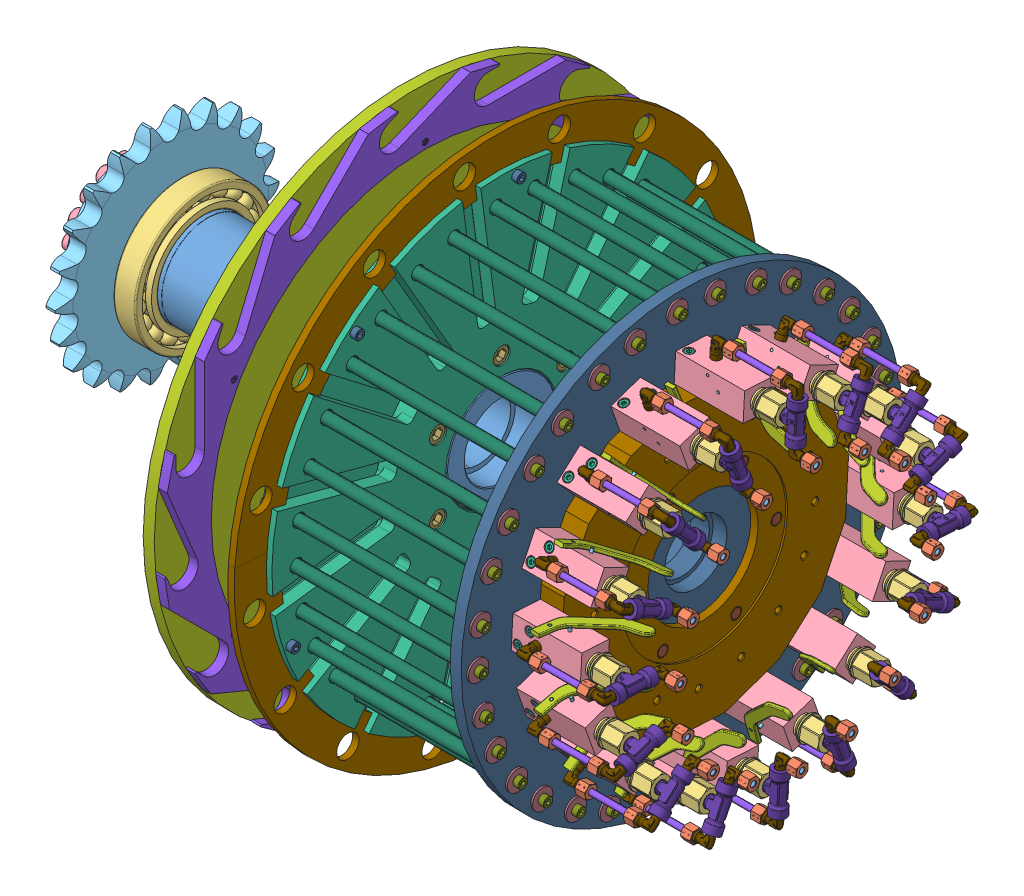
SolidWorks assembly Assieme1, configuration Default. Lengths in mm. (continued)
Components (placement in the parent): (continued)
- AssiemeValvola-7: AssiemeValvola [Default] at (515.3257 -134.8578 488.6421) x (0 0.901303 -0.433189) z (0 -0.433189 -0.901303) size (90.26 138.63 38)
  - RaccordoT-1: RaccordoT [Default] at origin size (43 29.75 16.5)
  - Raccordo a L-1: Raccordo a L [Default] at (-30 0 0) x (0 -1 0) z (0 0 -1) size (28.34 25.51 14.01)
    - 1809_06_10_01-1: 1809_06_10_01 [Default] at origin size (22.49 23 10)
    - 1809_06_10_02-1: 1809_06_10_02 [Default] at origin size (6.5 8.5 8.5)
    - 1809_06_10_03-1: 1809_06_10_03 [Default] at origin size (11.02 15.01 14.01)
  - Raccordo a L-2: Raccordo a L [Default] at (30 0 0) x (0 1 0) z (0 0 -1) size (28.34 25.51 14.01)
    - 1809_06_10_01-1: 1809_06_10_01 [Default] at origin size (22.49 23 10)
    - 1809_06_10_02-1: 1809_06_10_02 [Default] at origin size (6.5 8.5 8.5)
    - 1809_06_10_03-1: 1809_06_10_03 [Default] at origin size (11.02 15.01 14.01)
  - TappoChiusura-1: TappoChiusura [Default] at (0 -32 0) x (0 -1 0) z (0 0 1) size (38.28 26.74 26.74)
  - CorpoValvola-1: CorpoValvola [Default] at (-15 -115.2824 0) size (30 75 34)
  - Raccordo a L-3: Raccordo a L [Default] at (-30 -88.2824 0) x (0 1 0) z (0 0 1) size (28.34 25.51 14.01)
    - 1809_06_10_01-1: 1809_06_10_01 [Default] at origin size (22.49 23 10)
    - 1809_06_10_02-1: 1809_06_10_02 [Default] at origin size (6.5 8.5 8.5)
    - 1809_06_10_03-1: 1809_06_10_03 [Default] at origin size (11.02 15.01 14.01)
  - Spina_3x38-1: Spina_3x38 [Default] at (0 -68.2824 -21) x (-1 0 0) z (0 0 1) size (3 3 38)
  - Spina_3x38-2: Spina_3x38 [Default] at (-10 -80.2824 -21) x (0.996193 0.087174 0) z (0 0 1) size (3 3 38)
  - M5 40mm-3: M5 40mm [ISO 4762 M5 x 40 - 40N] at (-14.6 -108.7824 9) size (45 8.5 8.5)
  - M5 40mm-2: M5 40mm [ISO 4762 M5 x 40 - 40N] at (-14.6 -96.7824 -9) size (45 8.5 8.5)
  - LevaValvola-1: LevaValvola [Default] at (-24.507 -86.571 -17) x (0.996193 0.087174 0) z (0 0 1) size (77.55 60.2 4)
  - Tubo-1: Tubo [Default] at (-30 -15.9665 0) x (1 0 0) z (0 -1 0) size (6 6 56.4)
- AssiemeValvola-8: AssiemeValvola [Default] at (515.3257 -95.0129 541.6718) x (0 0.666921 -0.745128) z (0 -0.745128 -0.666921) size (90.26 138.63 38)
  - RaccordoT-1: RaccordoT [Default] at origin size (43 29.75 16.5)
  - Raccordo a L-1: Raccordo a L [Default] at (-30 0 0) x (0 -1 0) z (0 0 -1) size (28.34 25.51 14.01)
    - 1809_06_10_01-1: 1809_06_10_01 [Default] at origin size (22.49 23 10)
    - 1809_06_10_02-1: 1809_06_10_02 [Default] at origin size (6.5 8.5 8.5)
    - 1809_06_10_03-1: 1809_06_10_03 [Default] at origin size (11.02 15.01 14.01)
  - Raccordo a L-2: Raccordo a L [Default] at (30 0 0) x (0 1 0) z (0 0 -1) size (28.34 25.51 14.01)
    - 1809_06_10_01-1: 1809_06_10_01 [Default] at origin size (22.49 23 10)
    - 1809_06_10_02-1: 1809_06_10_02 [Default] at origin size (6.5 8.5 8.5)
    - 1809_06_10_03-1: 1809_06_10_03 [Default] at origin size (11.02 15.01 14.01)
  - TappoChiusura-1: TappoChiusura [Default] at (0 -32 0) x (0 -1 0) z (0 0 1) size (38.28 26.74 26.74)
  - CorpoValvola-1: CorpoValvola [Default] at (-15 -115.2824 0) size (30 75 34)
  - Raccordo a L-3: Raccordo a L [Default] at (-30 -88.2824 0) x (0 1 0) z (0 0 1) size (28.34 25.51 14.01)
    - 1809_06_10_01-1: 1809_06_10_01 [Default] at origin size (22.49 23 10)
    - 1809_06_10_02-1: 1809_06_10_02 [Default] at origin size (6.5 8.5 8.5)
    - 1809_06_10_03-1: 1809_06_10_03 [Default] at origin size (11.02 15.01 14.01)
  - Spina_3x38-1: Spina_3x38 [Default] at (0 -68.2824 -21) x (-1 0 0) z (0 0 1) size (3 3 38)
  - Spina_3x38-2: Spina_3x38 [Default] at (-10 -80.2824 -21) x (0.996193 0.087174 0) z (0 0 1) size (3 3 38)
  - M5 40mm-3: M5 40mm [ISO 4762 M5 x 40 - 40N] at (-14.6 -108.7824 9) size (45 8.5 8.5)
  - M5 40mm-2: M5 40mm [ISO 4762 M5 x 40 - 40N] at (-14.6 -96.7824 -9) size (45 8.5 8.5)
  - LevaValvola-1: LevaValvola [Default] at (-24.507 -86.571 -17) x (0.996193 0.087174 0) z (0 0 1) size (77.55 60.2 4)
  - Tubo-1: Tubo [Default] at (-30 -15.9665 0) x (1 0 0) z (0 -1 0) size (6 6 56.4)
- AssiemeValvola-9: AssiemeValvola [Default] at (515.3257 -37.9074 575.4168) x (0 0.331007 -0.943628) z (0 -0.943628 -0.331007) size (90.26 138.63 38)
  - RaccordoT-1: RaccordoT [Default] at origin size (43 29.75 16.5)
  - Raccordo a L-1: Raccordo a L [Default] at (-30 0 0) x (0 -1 0) z (0 0 -1) size (28.34 25.51 14.01)
    - 1809_06_10_01-1: 1809_06_10_01 [Default] at origin size (22.49 23 10)
    - 1809_06_10_02-1: 1809_06_10_02 [Default] at origin size (6.5 8.5 8.5)
    - 1809_06_10_03-1: 1809_06_10_03 [Default] at origin size (11.02 15.01 14.01)
  - Raccordo a L-2: Raccordo a L [Default] at (30 0 0) x (0 1 0) z (0 0 -1) size (28.34 25.51 14.01)
    - 1809_06_10_01-1: 1809_06_10_01 [Default] at origin size (22.49 23 10)
    - 1809_06_10_02-1: 1809_06_10_02 [Default] at origin size (6.5 8.5 8.5)
    - 1809_06_10_03-1: 1809_06_10_03 [Default] at origin size (11.02 15.01 14.01)
  - TappoChiusura-1: TappoChiusura [Default] at (0 -32 0) x (0 -1 0) z (0 0 1) size (38.28 26.74 26.74)
  - CorpoValvola-1: CorpoValvola [Default] at (-15 -115.2824 0) size (30 75 34)
  - Raccordo a L-3: Raccordo a L [Default] at (-30 -88.2824 0) x (0 1 0) z (0 0 1) size (28.34 25.51 14.01)
    - 1809_06_10_01-1: 1809_06_10_01 [Default] at origin size (22.49 23 10)
    - 1809_06_10_02-1: 1809_06_10_02 [Default] at origin size (6.5 8.5 8.5)
    - 1809_06_10_03-1: 1809_06_10_03 [Default] at origin size (11.02 15.01 14.01)
  - Spina_3x38-1: Spina_3x38 [Default] at (0 -68.2824 -21) x (-1 0 0) z (0 0 1) size (3 3 38)
  - Spina_3x38-2: Spina_3x38 [Default] at (-10 -80.2824 -21) x (0.996193 0.087174 0) z (0 0 1) size (3 3 38)
  - M5 40mm-3: M5 40mm [ISO 4762 M5 x 40 - 40N] at (-14.6 -108.7824 9) size (45 8.5 8.5)
  - M5 40mm-2: M5 40mm [ISO 4762 M5 x 40 - 40N] at (-14.6 -96.7824 -9) size (45 8.5 8.5)
  - LevaValvola-1: LevaValvola [Default] at (-24.507 -86.571 -17) x (0.996193 0.087174 0) z (0 0 1) size (77.55 60.2 4)
  - Tubo-1: Tubo [Default] at (-30 -15.9665 0) x (1 0 0) z (0 -1 0) size (6 6 56.4)
- AssiemeValvola-10: AssiemeValvola [Default] at (515.3257 27.7648 584.7399) x (0 -0.055301 -0.99847) z (0 -0.99847 0.055301) size (90.26 138.63 38)
  - RaccordoT-1: RaccordoT [Default] at origin size (43 29.75 16.5)
  - Raccordo a L-1: Raccordo a L [Default] at (-30 0 0) x (0 -1 0) z (0 0 -1) size (28.34 25.51 14.01)
    - 1809_06_10_01-1: 1809_06_10_01 [Default] at origin size (22.49 23 10)
    - 1809_06_10_02-1: 1809_06_10_02 [Default] at origin size (6.5 8.5 8.5)
    - 1809_06_10_03-1: 1809_06_10_03 [Default] at origin size (11.02 15.01 14.01)
  - Raccordo a L-2: Raccordo a L [Default] at (30 0 0) x (0 1 0) z (0 0 -1) size (28.34 25.51 14.01)
    - 1809_06_10_01-1: 1809_06_10_01 [Default] at origin size (22.49 23 10)
    - 1809_06_10_02-1: 1809_06_10_02 [Default] at origin size (6.5 8.5 8.5)
    - 1809_06_10_03-1: 1809_06_10_03 [Default] at origin size (11.02 15.01 14.01)
  - TappoChiusura-1: TappoChiusura [Default] at (0 -32 0) x (0 -1 0) z (0 0 1) size (38.28 26.74 26.74)
  - CorpoValvola-1: CorpoValvola [Default] at (-15 -115.2824 0) size (30 75 34)
  - Raccordo a L-3: Raccordo a L [Default] at (-30 -88.2824 0) x (0 1 0) z (0 0 1) size (28.34 25.51 14.01)
    - 1809_06_10_01-1: 1809_06_10_01 [Default] at origin size (22.49 23 10)
    - 1809_06_10_02-1: 1809_06_10_02 [Default] at origin size (6.5 8.5 8.5)
    - 1809_06_10_03-1: 1809_06_10_03 [Default] at origin size (11.02 15.01 14.01)
  - Spina_3x38-1: Spina_3x38 [Default] at (0 -68.2824 -21) x (-1 0 0) z (0 0 1) size (3 3 38)
  - Spina_3x38-2: Spina_3x38 [Default] at (-10 -80.2824 -21) x (0.996193 0.087174 0) z (0 0 1) size (3 3 38)
  - M5 40mm-3: M5 40mm [ISO 4762 M5 x 40 - 40N] at (-14.6 -108.7824 9) size (45 8.5 8.5)
  - M5 40mm-2: M5 40mm [ISO 4762 M5 x 40 - 40N] at (-14.6 -96.7824 -9) size (45 8.5 8.5)
  - LevaValvola-1: LevaValvola [Default] at (-24.507 -86.571 -17) x (0.996193 0.087174 0) z (0 0 1) size (77.55 60.2 4)
  - Tubo-1: Tubo [Default] at (-30 -15.9665 0) x (1 0 0) z (0 -1 0) size (6 6 56.4)
- AssiemeValvola-11: AssiemeValvola [Default] at (515.3257 92.0058 568.2215) x (0 -0.433189 -0.901303) z (0 -0.901303 0.433189) size (90.26 138.63 38)
  - RaccordoT-1: RaccordoT [Default] at origin size (43 29.75 16.5)
  - Raccordo a L-1: Raccordo a L [Default] at (-30 0 0) x (0 -1 0) z (0 0 -1) size (28.34 25.51 14.01)
    - 1809_06_10_01-1: 1809_06_10_01 [Default] at origin size (22.49 23 10)
    - 1809_06_10_02-1: 1809_06_10_02 [Default] at origin size (6.5 8.5 8.5)
    - 1809_06_10_03-1: 1809_06_10_03 [Default] at origin size (11.02 15.01 14.01)
  - Raccordo a L-2: Raccordo a L [Default] at (30 0 0) x (0 1 0) z (0 0 -1) size (28.34 25.51 14.01)
    - 1809_06_10_01-1: 1809_06_10_01 [Default] at origin size (22.49 23 10)
    - 1809_06_10_02-1: 1809_06_10_02 [Default] at origin size (6.5 8.5 8.5)
    - 1809_06_10_03-1: 1809_06_10_03 [Default] at origin size (11.02 15.01 14.01)
  - TappoChiusura-1: TappoChiusura [Default] at (0 -32 0) x (0 -1 0) z (0 0 1) size (38.28 26.74 26.74)
  - CorpoValvola-1: CorpoValvola [Default] at (-15 -115.2824 0) size (30 75 34)
  - Raccordo a L-3: Raccordo a L [Default] at (-30 -88.2824 0) x (0 1 0) z (0 0 1) size (28.34 25.51 14.01)
    - 1809_06_10_01-1: 1809_06_10_01 [Default] at origin size (22.49 23 10)
    - 1809_06_10_02-1: 1809_06_10_02 [Default] at origin size (6.5 8.5 8.5)
    - 1809_06_10_03-1: 1809_06_10_03 [Default] at origin size (11.02 15.01 14.01)
  - Spina_3x38-1: Spina_3x38 [Default] at (0 -68.2824 -21) x (-1 0 0) z (0 0 1) size (3 3 38)
  - Spina_3x38-2: Spina_3x38 [Default] at (-10 -80.2824 -21) x (0.996193 0.087174 0) z (0 0 1) size (3 3 38)
  - M5 40mm-3: M5 40mm [ISO 4762 M5 x 40 - 40N] at (-14.6 -108.7824 9) size (45 8.5 8.5)
  - M5 40mm-2: M5 40mm [ISO 4762 M5 x 40 - 40N] at (-14.6 -96.7824 -9) size (45 8.5 8.5)
  - LevaValvola-1: LevaValvola [Default] at (-24.507 -86.571 -17) x (0.996193 0.087174 0) z (0 0 1) size (77.55 60.2 4)
  - Tubo-1: Tubo [Default] at (-30 -15.9665 0) x (1 0 0) z (0 -1 0) size (6 6 56.4)
- AssiemeValvola-12: AssiemeValvola [Default] at (515.3257 145.0355 528.3766) x (0 -0.745128 -0.666921) z (0 -0.666921 0.745128) size (90.26 138.63 38)
  - RaccordoT-1: RaccordoT [Default] at origin size (43 29.75 16.5)
  - Raccordo a L-1: Raccordo a L [Default] at (-30 0 0) x (0 -1 0) z (0 0 -1) size (28.34 25.51 14.01)
    - 1809_06_10_01-1: 1809_06_10_01 [Default] at origin size (22.49 23 10)
    - 1809_06_10_02-1: 1809_06_10_02 [Default] at origin size (6.5 8.5 8.5)
    - 1809_06_10_03-1: 1809_06_10_03 [Default] at origin size (11.02 15.01 14.01)
  - Raccordo a L-2: Raccordo a L [Default] at (30 0 0) x (0 1 0) z (0 0 -1) size (28.34 25.51 14.01)
    - 1809_06_10_01-1: 1809_06_10_01 [Default] at origin size (22.49 23 10)
    - 1809_06_10_02-1: 1809_06_10_02 [Default] at origin size (6.5 8.5 8.5)
    - 1809_06_10_03-1: 1809_06_10_03 [Default] at origin size (11.02 15.01 14.01)
  - TappoChiusura-1: TappoChiusura [Default] at (0 -32 0) x (0 -1 0) z (0 0 1) size (38.28 26.74 26.74)
  - CorpoValvola-1: CorpoValvola [Default] at (-15 -115.2824 0) size (30 75 34)
  - Raccordo a L-3: Raccordo a L [Default] at (-30 -88.2824 0) x (0 1 0) z (0 0 1) size (28.34 25.51 14.01)
    - 1809_06_10_01-1: 1809_06_10_01 [Default] at origin size (22.49 23 10)
    - 1809_06_10_02-1: 1809_06_10_02 [Default] at origin size (6.5 8.5 8.5)
    - 1809_06_10_03-1: 1809_06_10_03 [Default] at origin size (11.02 15.01 14.01)
  - Spina_3x38-1: Spina_3x38 [Default] at (0 -68.2824 -21) x (-1 0 0) z (0 0 1) size (3 3 38)
  - Spina_3x38-2: Spina_3x38 [Default] at (-10 -80.2824 -21) x (0.996193 0.087174 0) z (0 0 1) size (3 3 38)
  - M5 40mm-3: M5 40mm [ISO 4762 M5 x 40 - 40N] at (-14.6 -108.7824 9) size (45 8.5 8.5)
  - M5 40mm-2: M5 40mm [ISO 4762 M5 x 40 - 40N] at (-14.6 -96.7824 -9) size (45 8.5 8.5)
  - LevaValvola-1: LevaValvola [Default] at (-24.507 -86.571 -17) x (0.996193 0.087174 0) z (0 0 1) size (77.55 60.2 4)
  - Tubo-1: Tubo [Default] at (-30 -15.9665 0) x (1 0 0) z (0 -1 0) size (6 6 56.4)
- AssiemeValvola-13: AssiemeValvola [Default] at (515.3257 178.7805 471.2711) x (0 -0.943628 -0.331007) z (0 -0.331007 0.943628) size (90.26 138.63 38)
  - RaccordoT-1: RaccordoT [Default] at origin size (43 29.75 16.5)
  - Raccordo a L-1: Raccordo a L [Default] at (-30 0 0) x (0 -1 0) z (0 0 -1) size (28.34 25.51 14.01)
    - 1809_06_10_01-1: 1809_06_10_01 [Default] at origin size (22.49 23 10)
    - 1809_06_10_02-1: 1809_06_10_02 [Default] at origin size (6.5 8.5 8.5)
    - 1809_06_10_03-1: 1809_06_10_03 [Default] at origin size (11.02 15.01 14.01)
  - Raccordo a L-2: Raccordo a L [Default] at (30 0 0) x (0 1 0) z (0 0 -1) size (28.34 25.51 14.01)
    - 1809_06_10_01-1: 1809_06_10_01 [Default] at origin size (22.49 23 10)
    - 1809_06_10_02-1: 1809_06_10_02 [Default] at origin size (6.5 8.5 8.5)
    - 1809_06_10_03-1: 1809_06_10_03 [Default] at origin size (11.02 15.01 14.01)
  - TappoChiusura-1: TappoChiusura [Default] at (0 -32 0) x (0 -1 0) z (0 0 1) size (38.28 26.74 26.74)
  - CorpoValvola-1: CorpoValvola [Default] at (-15 -115.2824 0) size (30 75 34)
  - Raccordo a L-3: Raccordo a L [Default] at (-30 -88.2824 0) x (0 1 0) z (0 0 1) size (28.34 25.51 14.01)
    - 1809_06_10_01-1: 1809_06_10_01 [Default] at origin size (22.49 23 10)
    - 1809_06_10_02-1: 1809_06_10_02 [Default] at origin size (6.5 8.5 8.5)
    - 1809_06_10_03-1: 1809_06_10_03 [Default] at origin size (11.02 15.01 14.01)
  - Spina_3x38-1: Spina_3x38 [Default] at (0 -68.2824 -21) x (-1 0 0) z (0 0 1) size (3 3 38)
  - Spina_3x38-2: Spina_3x38 [Default] at (-10 -80.2824 -21) x (0.996193 0.087174 0) z (0 0 1) size (3 3 38)
  - M5 40mm-3: M5 40mm [ISO 4762 M5 x 40 - 40N] at (-14.6 -108.7824 9) size (45 8.5 8.5)
  - M5 40mm-2: M5 40mm [ISO 4762 M5 x 40 - 40N] at (-14.6 -96.7824 -9) size (45 8.5 8.5)
  - LevaValvola-1: LevaValvola [Default] at (-24.507 -86.571 -17) x (0.996193 0.087174 0) z (0 0 1) size (77.55 60.2 4)
  - Tubo-1: Tubo [Default] at (-30 -15.9665 0) x (1 0 0) z (0 -1 0) size (6 6 56.4)
- AssiemeValvola-14: AssiemeValvola [Default] at (515.3257 188.1036 405.5989) x (0 -0.99847 0.055301) z (0 0.055301 0.99847) size (90.26 138.63 38)
  - RaccordoT-1: RaccordoT [Default] at origin size (43 29.75 16.5)
  - Raccordo a L-1: Raccordo a L [Default] at (-30 0 0) x (0 -1 0) z (0 0 -1) size (28.34 25.51 14.01)
    - 1809_06_10_01-1: 1809_06_10_01 [Default] at origin size (22.49 23 10)
    - 1809_06_10_02-1: 1809_06_10_02 [Default] at origin size (6.5 8.5 8.5)
    - 1809_06_10_03-1: 1809_06_10_03 [Default] at origin size (11.02 15.01 14.01)
  - Raccordo a L-2: Raccordo a L [Default] at (30 0 0) x (0 1 0) z (0 0 -1) size (28.34 25.51 14.01)
    - 1809_06_10_01-1: 1809_06_10_01 [Default] at origin size (22.49 23 10)
    - 1809_06_10_02-1: 1809_06_10_02 [Default] at origin size (6.5 8.5 8.5)
    - 1809_06_10_03-1: 1809_06_10_03 [Default] at origin size (11.02 15.01 14.01)
  - TappoChiusura-1: TappoChiusura [Default] at (0 -32 0) x (0 -1 0) z (0 0 1) size (38.28 26.74 26.74)
  - CorpoValvola-1: CorpoValvola [Default] at (-15 -115.2824 0) size (30 75 34)
  - Raccordo a L-3: Raccordo a L [Default] at (-30 -88.2824 0) x (0 1 0) z (0 0 1) size (28.34 25.51 14.01)
    - 1809_06_10_01-1: 1809_06_10_01 [Default] at origin size (22.49 23 10)
    - 1809_06_10_02-1: 1809_06_10_02 [Default] at origin size (6.5 8.5 8.5)
    - 1809_06_10_03-1: 1809_06_10_03 [Default] at origin size (11.02 15.01 14.01)
  - Spina_3x38-1: Spina_3x38 [Default] at (0 -68.2824 -21) x (-1 0 0) z (0 0 1) size (3 3 38)
  - Spina_3x38-2: Spina_3x38 [Default] at (-10 -80.2824 -21) x (0.996193 0.087174 0) z (0 0 1) size (3 3 38)
  - M5 40mm-3: M5 40mm [ISO 4762 M5 x 40 - 40N] at (-14.6 -108.7824 9) size (45 8.5 8.5)
  - M5 40mm-2: M5 40mm [ISO 4762 M5 x 40 - 40N] at (-14.6 -96.7824 -9) size (45 8.5 8.5)
  - LevaValvola-1: LevaValvola [Default] at (-24.507 -86.571 -17) x (0.996193 0.087174 0) z (0 0 1) size (77.55 60.2 4)
  - Tubo-1: Tubo [Default] at (-30 -15.9665 0) x (1 0 0) z (0 -1 0) size (6 6 56.4)
- AssiemeValvola-15: AssiemeValvola [Default] at (515.3257 171.5852 341.3579) x (0 -0.901303 0.433189) z (0 0.433189 0.901303) size (90.26 138.63 38)
  - RaccordoT-1: RaccordoT [Default] at origin size (43 29.75 16.5)
  - Raccordo a L-1: Raccordo a L [Default] at (-30 0 0) x (0 -1 0) z (0 0 -1) size (28.34 25.51 14.01)
    - 1809_06_10_01-1: 1809_06_10_01 [Default] at origin size (22.49 23 10)
    - 1809_06_10_02-1: 1809_06_10_02 [Default] at origin size (6.5 8.5 8.5)
    - 1809_06_10_03-1: 1809_06_10_03 [Default] at origin size (11.02 15.01 14.01)
  - Raccordo a L-2: Raccordo a L [Default] at (30 0 0) x (0 1 0) z (0 0 -1) size (28.34 25.51 14.01)
    - 1809_06_10_01-1: 1809_06_10_01 [Default] at origin size (22.49 23 10)
    - 1809_06_10_02-1: 1809_06_10_02 [Default] at origin size (6.5 8.5 8.5)
    - 1809_06_10_03-1: 1809_06_10_03 [Default] at origin size (11.02 15.01 14.01)
  - TappoChiusura-1: TappoChiusura [Default] at (0 -32 0) x (0 -1 0) z (0 0 1) size (38.28 26.74 26.74)
  - CorpoValvola-1: CorpoValvola [Default] at (-15 -115.2824 0) size (30 75 34)
  - Raccordo a L-3: Raccordo a L [Default] at (-30 -88.2824 0) x (0 1 0) z (0 0 1) size (28.34 25.51 14.01)
    - 1809_06_10_01-1: 1809_06_10_01 [Default] at origin size (22.49 23 10)
    - 1809_06_10_02-1: 1809_06_10_02 [Default] at origin size (6.5 8.5 8.5)
    - 1809_06_10_03-1: 1809_06_10_03 [Default] at origin size (11.02 15.01 14.01)
  - Spina_3x38-1: Spina_3x38 [Default] at (0 -68.2824 -21) x (-1 0 0) z (0 0 1) size (3 3 38)
  - Spina_3x38-2: Spina_3x38 [Default] at (-10 -80.2824 -21) x (0.996193 0.087174 0) z (0 0 1) size (3 3 38)
  - M5 40mm-3: M5 40mm [ISO 4762 M5 x 40 - 40N] at (-14.6 -108.7824 9) size (45 8.5 8.5)
  - M5 40mm-2: M5 40mm [ISO 4762 M5 x 40 - 40N] at (-14.6 -96.7824 -9) size (45 8.5 8.5)
  - LevaValvola-1: LevaValvola [Default] at (-24.507 -86.571 -17) x (0.996193 0.087174 0) z (0 0 1) size (77.55 60.2 4)
  - Tubo-1: Tubo [Default] at (-30 -15.9665 0) x (1 0 0) z (0 -1 0) size (6 6 56.4)
- AssiemeValvola-16: AssiemeValvola [Default] at (515.3257 131.7403 288.3282) x (0 -0.666921 0.745128) z (0 0.745128 0.666921) size (90.26 138.63 38)
  - RaccordoT-1: RaccordoT [Default] at origin size (43 29.75 16.5)
  - Raccordo a L-1: Raccordo a L [Default] at (-30 0 0) x (0 -1 0) z (0 0 -1) size (28.34 25.51 14.01)
    - 1809_06_10_01-1: 1809_06_10_01 [Default] at origin size (22.49 23 10)
    - 1809_06_10_02-1: 1809_06_10_02 [Default] at origin size (6.5 8.5 8.5)
    - 1809_06_10_03-1: 1809_06_10_03 [Default] at origin size (11.02 15.01 14.01)
  - Raccordo a L-2: Raccordo a L [Default] at (30 0 0) x (0 1 0) z (0 0 -1) size (28.34 25.51 14.01)
    - 1809_06_10_01-1: 1809_06_10_01 [Default] at origin size (22.49 23 10)
    - 1809_06_10_02-1: 1809_06_10_02 [Default] at origin size (6.5 8.5 8.5)
    - 1809_06_10_03-1: 1809_06_10_03 [Default] at origin size (11.02 15.01 14.01)
  - TappoChiusura-1: TappoChiusura [Default] at (0 -32 0) x (0 -1 0) z (0 0 1) size (38.28 26.74 26.74)
  - CorpoValvola-1: CorpoValvola [Default] at (-15 -115.2824 0) size (30 75 34)
  - Raccordo a L-3: Raccordo a L [Default] at (-30 -88.2824 0) x (0 1 0) z (0 0 1) size (28.34 25.51 14.01)
    - 1809_06_10_01-1: 1809_06_10_01 [Default] at origin size (22.49 23 10)
    - 1809_06_10_02-1: 1809_06_10_02 [Default] at origin size (6.5 8.5 8.5)
    - 1809_06_10_03-1: 1809_06_10_03 [Default] at origin size (11.02 15.01 14.01)
  - Spina_3x38-1: Spina_3x38 [Default] at (0 -68.2824 -21) x (-1 0 0) z (0 0 1) size (3 3 38)
  - Spina_3x38-2: Spina_3x38 [Default] at (-10 -80.2824 -21) x (0.996193 0.087174 0) z (0 0 1) size (3 3 38)
  - M5 40mm-3: M5 40mm [ISO 4762 M5 x 40 - 40N] at (-14.6 -108.7824 9) size (45 8.5 8.5)
  - M5 40mm-2: M5 40mm [ISO 4762 M5 x 40 - 40N] at (-14.6 -96.7824 -9) size (45 8.5 8.5)
  - LevaValvola-1: LevaValvola [Default] at (-24.507 -86.571 -17) x (0.996193 0.087174 0) z (0 0 1) size (77.55 60.2 4)
  - Tubo-1: Tubo [Default] at (-30 -15.9665 0) x (1 0 0) z (0 -1 0) size (6 6 56.4)
- Disco alimentazione guarnizione fi24.4-1: Disco alimentazione guarnizione fi24.4 [Default] at (198.0433 18.3637 415) x (0 0.065403 0.997859) z (-1 0 0) size (570 285 7.35)
- Disco alimentazione guarnizione fi24.4-2: Disco alimentazione guarnizione fi24.4 [Default] at (198.0433 18.3637 415) x (0 -0.065403 -0.997859) z (-1 0 0) size (570 285 7.35)
- m6 12mm-1: m6 12mm [ISO 4762 M6 x 12 - 12N] at (210.0433 200.6849 574.8914) x (-1 0 0) z (0 0.793353 -0.608761) size (18 10 10)
- m6 12mm-7: m6 12mm [ISO 4762 M6 x 12 - 12N] at (210.0433 260.3445 399.1397) x (-1 0 0) z (0 0.793353 -0.608761) size (18 10 10)
- m6 12mm-8: m6 12mm [ISO 4762 M6 x 12 - 12N] at (210.0433 96.3128 185.3694) x (-1 0 0) z (0 0.793353 -0.608761) size (18 10 10)
- m6 12mm-9: m6 12mm [ISO 4762 M6 x 12 - 12N] at (210.0433 -59.5854 644.6306) x (-1 0 0) z (0 -0.793353 -0.608761) size (18 10 10)
- m6 12mm-10: m6 12mm [ISO 4762 M6 x 12 - 12N] at (210.0433 -223.6171 430.8603) x (-1 0 0) z (0 -0.793353 -0.608761) size (18 10 10)
- m6 12mm-11: m6 12mm [ISO 4762 M6 x 12 - 12N] at (210.0433 -163.9575 255.1086) x (-1 0 0) z (0 0.793353 -0.608761) size (18 10 10)
Mates (geometry in assembly coordinates):
- Concentrico1: concentric anti-aligned: circle of albero rotazione piatti-1; circle of seger 100mm-1
- Coincidente1: coincident anti-aligned: plane of albero rotazione piatti-1 through (-143.4567 18.3637 415) normal (-1 0 0); plane of seger 100mm-1 through (-143.4567 18.3637 415) normal (1 0 0)
- Coincidente2: coincident aligned: plane of albero rotazione piatti-1 through (60.413 18.3637 415) normal (0 1 0); plane of seger 100mm-1 through (-146.4567 18.3637 415) normal (0 1 0)
- Concentrico21: concentric aligned: cylinder of albero rotazione piatti-1 through (60.413 18.3637 415) axis (1 0 0) radius 50; cylinder of SKF - 6020 - 20,DE,NC,20_68-1 through (-152.0942 18.3637 415) axis (1 0 0) radius 50
- Coincidente3: coincident anti-aligned: plane of seger 100mm-1 through (-143.4567 18.3637 415) normal (1 0 0); plane of SKF - 6020 - 20,DE,NC,20_68-1 through (-143.4567 -33.4256 439.9823) normal (-1 0 0)
- Concentrico3: concentric aligned: cylinder of albero rotazione piatti-1 through (60.413 18.3637 415) axis (1 0 0) radius 47.5; cylinder of calettatore d95-1 through (-199.9572 18.3637 415) axis (1 0 0) radius 47.5
- Concentrico4: concentric anti-aligned: cylinder of calettatore d95-1 through (-196.9572 18.3637 415) axis (1 0 0) radius 67.5; cylinder of pulegia z =50-1 through (-170.9572 18.3637 415) axis (-1 0 0) radius 67.5
- Coincidente4: coincident anti-aligned: plane of calettatore d95-1 through (-170.9572 84.9137 415) normal (1 0 0); plane of pulegia z =50-1 through (-170.9572 18.3637 415) normal (-1 0 0)
- Coincidente5: coincident anti-aligned: plane of albero rotazione piatti-1 through (-155.9567 18.3637 415) normal (-1 0 0); plane of pulegia z =50-1 through (-155.9567 18.3637 415) normal (1 0 0)
- Coincidente6: coincident aligned: plane of calettatore d95-1 through (-184.9572 18.3637 415) normal (0 1 0); plane of pulegia z =50-1 through (-173.9167 18.3637 415) normal (0 1 0)
- Coincidente7: coincident aligned: plane of albero rotazione piatti-1 through (60.413 18.3637 415) normal (0 1 0); plane of calettatore d95-1 through (-184.9572 18.3637 415) normal (0 1 0)
- Concentrico5: concentric aligned: cylinder of albero rotazione piatti-1 through (60.413 18.3637 415) axis (1 0 0) radius 49.75; cylinder of SKF - 6020 - 20,DE,NC,20_68-2 through (41.4058 18.3637 415) axis (1 0 0) radius 50
- Coincidente8: coincident anti-aligned: plane of albero rotazione piatti-1 through (74.0433 18.3637 415) normal (-1 0 0); plane of SKF - 6020 - 20,DE,NC,20_68-2 through (74.0433 -28.0673 437.2803) normal (1 0 0)
- Concentrico6: concentric aligned: cylinder of albero rotazione piatti-1 through (60.413 18.3637 415) axis (1 0 0) radius 60; cylinder of Disco supporto montaggio e Colonne-1 through (5.3377 18.3637 415) axis (1 0 0) radius 60
- Concentrico7: concentric aligned: cylinder of albero rotazione piatti-1 through (101.3656 98.3637 415) axis (1 0 0) radius 6.25; cylinder of Disco supporto montaggio e Colonne-1 through (204.0433 98.3637 415) axis (1 0 0) radius 9.25
- Coincidente9: coincident anti-aligned: plane of albero rotazione piatti-1 through (175.0433 18.3637 415) normal (1 0 0); plane of Disco supporto montaggio e Colonne-1 through (175.0433 18.3637 415) normal (-1 0 0)
- Concentrico8: concentric anti-aligned: cylinder of albero rotazione piatti-1 through (60.413 18.3637 415) axis (1 0 0) radius 60; cylinder of piatto rotante porta tappi-1 through (111.0433 18.3637 415) axis (-1 0 0) radius 60
- Concentrico9: concentric aligned: circle of albero rotazione piatti-1; circle of piatto rotante porta tappi-1
- Coincidente10: coincident anti-aligned: plane of albero rotazione piatti-1 through (119.0433 18.3637 415) normal (-1 0 0); plane of piatto rotante porta tappi-1 through (119.0433 18.3637 415) normal (1 0 0)
- Concentrico10: concentric aligned: cylinder of piatto rotante porta tappi-1 through (119.0433 18.3637 415) axis (-1 0 0) radius 233; cylinder of disco trasportatore tappi 31-1 through (121.0433 18.3637 415) axis (-1 0 0) radius 233
- Tangente2: tangent: cylinder of piatto rotante porta tappi-1 through (98.5243 -101.6363 622.8461) axis (1 0 0) radius 3.25; curve of disco trasportatore tappi 31-1
- Coincidente13: coincident anti-aligned: plane of piatto rotante porta tappi-1 through (111.0433 18.3637 415) normal (1 0 0); plane of disco trasportatore tappi 31-1 through (111.0433 18.3637 415) normal (-1 0 0)
- Concentrico11: concentric anti-aligned: cylinder of albero rotazione piatti-1 through (60.413 18.3637 415) axis (1 0 0) radius 40; cylinder of disco trascinato porta distributore vuoto-1 through (400.0433 18.3637 415) axis (-1 0 0) radius 30
- Concentrico12: concentric anti-aligned: cylinder of Disco supporto montaggio e Colonne-1 through (204.0433 -202.0247 450.2415) axis (1 0 0) radius 6; cylinder of disco trascinato porta distributore vuoto-1 through (417.0139 -202.0247 450.2415) axis (-1 0 0) radius 6
- Coincidente14: coincident anti-aligned: plane of Distributore Rotante-1 through (400.0433 18.3637 415) normal (-1 0 0); plane of disco trascinato porta distributore vuoto-1 through (400.0433 18.3637 415) normal (1 0 0)
- Concentrico13: concentric anti-aligned: circle of Distributore Rotante-1; circle of disco trascinato porta distributore vuoto-1
- Concentrico14: concentric anti-aligned: cylinder of Distributore Rotante-1 through (230.3377 18.3637 415) axis (1 0 0) radius 60; cylinder of disco trascinato porta distributore vuoto-1 through (415.0433 18.3637 415) axis (-1 0 0) radius 67.5
- Concentrico15: concentric anti-aligned: cylinder of disco trascinato porta distributore vuoto-1 through (388.0433 -53.0243 378.8925) axis (1 0 0) radius 6.25; cylinder of m12 35mm-1 through (344.2933 -53.0243 378.8925) axis (-1 0 0) radius 6
- Coincidente15: coincident anti-aligned: plane of disco trascinato porta distributore vuoto-1 through (388.0433 18.3637 415) normal (-1 0 0); plane of m12 35mm-1 through (388.0433 -45.2301 383.3925) normal (1 0 0)
- Parallelo1: parallel anti-aligned: plane of m12 35mm-1 through (382.0433 -47.9668 381.8125) normal (0 -1 0)
- Concentrico16: concentric aligned: cylinder of Disco supporto montaggio e Colonne-1 through (204.0433 -21.6363 345.718) axis (1 0 0) radius 9.25; cylinder of m12 90mm-3 through (234.7933 -21.6363 345.718) axis (1 0 0) radius 6
- Coincidente17: coincident anti-aligned: plane of Disco supporto montaggio e Colonne-1 through (191.0433 -27.049 342.593) normal (1 0 0); plane of m12 90mm-3 through (191.0433 -29.4305 341.218) normal (-1 0 0)
- Parallelo2: parallel aligned: plane of m12 35mm-1 through (382.0433 -47.9668 381.8125) normal (0 -1 0); plane of m12 90mm-3 through (197.0433 -16.5788 348.6379) normal (0 -1 0)
- Concentrico171: concentric anti-aligned: cylinder of piatto rotante porta tappi-1 through (98.5243 -101.6363 207.1539) axis (1 0 0) radius 3.25; cylinder of rondella m6 22mm-1 through (64.1183 -101.6363 207.1539) axis (-1 0 0) radius 3.3
- Coincidente191: coincident anti-aligned: plane of piatto rotante porta tappi-1 through (99.0433 18.3637 415) normal (-1 0 0); plane of rondella m6 22mm-1 through (99.0433 -101.6363 210.4539) normal (1 0 0)
- Parallelo3: parallel anti-aligned: plane of rondella m6 22mm-1 through (99.0433 -101.6363 207.1539) normal (0 -1 0)
- Concentrico181: concentric aligned: cylinder of rondella m6 22mm-1 through (64.1183 -101.6363 207.1539) axis (-1 0 0) radius 3.3; cylinder of M6 20mm-1 through (59.2933 -101.6363 207.1539) axis (-1 0 0) radius 5
- Coincidente211: coincident anti-aligned: plane of rondella m6 22mm-1 through (97.0433 -101.6363 218.1539) normal (-1 0 0); plane of M6 20mm-1 through (97.0433 -97.3062 204.6539) normal (1 0 0)
- Parallelo4: parallel aligned: plane of m12 35mm-1 through (382.0433 -47.9668 381.8125) normal (0 -0.5 -0.866025); plane of M6 20mm-1 through (94.0433 -101.6363 210.0892) normal (0 -0.5 -0.866025)
- Concentrico19: concentric anti-aligned: cylinder of Disco supporto montaggio e Colonne-1 through (204.0433 70.1437 197.9013) axis (1 0 0) radius 6; cylinder of asta scorrimento carello-1 through (400.0433 70.1437 197.9013) axis (-1 0 0) radius 6
- Concentrico201: concentric aligned: cylinder of asta scorrimento carello-1 through (175.0433 70.1437 197.9013) axis (-1 0 0) radius 3.2; cylinder of rondella m6 22mm-7 through (140.1183 70.1437 197.9013) axis (-1 0 0) radius 3.3
- Coincidente231: coincident anti-aligned: plane of asta scorrimento carello-1 through (175.0433 70.1437 197.9013) normal (-1 0 0); plane of rondella m6 22mm-7 through (175.0433 70.1437 201.2013) normal (1 0 0)
- Concentrico211: concentric aligned: cylinder of rondella m6 22mm-7 through (140.1183 70.1437 197.9013) axis (-1 0 0) radius 3.3; cylinder of M6 16mm-1 through (135.2933 70.1437 197.9013) axis (-1 0 0) radius 5
- Coincidente241: coincident anti-aligned: plane of rondella m6 22mm-7 through (173.0433 70.1437 208.9013) normal (-1 0 0); plane of M6 16mm-1 through (173.0433 75.1437 197.9013) normal (1 0 0)
- Parallelo5: parallel aligned: plane of asta scorrimento carello-1 through (287.5433 70.1437 197.9013) normal (0 0 -1); plane of M6 16mm-1 through (170.0433 68.6761 200.4433) normal (0 0 -1)
- Parallelo9: parallel anti-aligned: plane of rondella m6 22mm-7 through (175.0433 70.1437 197.9013) normal (0 0 1); plane of M6 16mm-1 through (170.0433 68.6761 200.4433) normal (0 0 -1)
- Coincidente30: coincident anti-aligned: plane of Disco supporto montaggio e Colonne-1 through (175.0433 18.3637 415) normal (-1 0 0); plane of rondella m6 22mm-7 through (175.0433 70.1437 201.2013) normal (1 0 0)
- Coincidente31: coincident anti-aligned: plane of disco trascinato porta distributore vuoto-1 through (400.0433 18.3637 415) normal (1 0 0); plane of rondella m6 22mm-8 through (400.0433 70.1437 201.2013) normal (-1 0 0)
- Coincidente32: coincident anti-aligned: plane of Distributore Rotante-1 through (400.0433 40.5763 258.5322) normal (0 0.331007 -0.943628); plane of AssiemeValvola-1/CorpoValvola-1 through (400.0433 85.7114 274.3647) normal (0 -0.331007 0.943628)
- Coincidente33: coincident anti-aligned: plane of disco trascinato porta distributore vuoto-1 through (400.0433 18.3637 415) normal (1 0 0); plane of AssiemeValvola-1/CorpoValvola-1 through (400.0433 95.6416 246.0559) normal (-1 0 0)
- Concentrico22: concentric anti-aligned: cylinder of Distributore Rotante-1 through (412.5433 55.4365 309.3136) axis (0 0.331007 -0.943628) radius 3; cylinder of AssiemeValvola-1/CorpoValvola-1 through (412.5433 69.6697 268.7376) axis (0 -0.331007 0.943628) radius 3
- Concentrico23: concentric anti-aligned: cylinder of Disco supporto montaggio e Colonne-1 through (198.0433 18.3637 415) axis (-1 0 0) radius 235; cylinder of Disco alimentazione guarnizione fi24.4-2 through (191.0433 18.3637 415) axis (1 0 0) radius 235
- Concentrico24: concentric anti-aligned: cylinder of Disco supporto montaggio e Colonne-1 through (198.0433 18.3637 415) axis (-1 0 0) radius 235; cylinder of Disco alimentazione guarnizione fi24.4-1 through (191.0433 18.3637 415) axis (1 0 0) radius 235
- Coincidente34: coincident anti-aligned: plane of Disco alimentazione guarnizione fi24.4-1 through (191.0433 33.7334 649.4968) normal (0 -0.997859 0.065403); plane of Disco alimentazione guarnizione fi24.4-2 through (191.0433 37.0036 699.3898) normal (0 0.997859 -0.065403)
- Coincidente35: coincident aligned: plane of Disco alimentazione guarnizione fi24.4-1 through (198.0433 18.3637 415) normal (1 0 0); plane of Disco alimentazione guarnizione fi24.4-2 through (198.0433 18.3637 415) normal (1 0 0)
- Concentrico25: concentric anti-aligned: cylinder of Disco supporto montaggio e Colonne-1 through (188.8509 -59.5854 644.6306) axis (1 0 0) radius 3.25; circle of Disco alimentazione guarnizione fi24.4-2
- Coincidente36: coincident anti-aligned: plane of Disco supporto montaggio e Colonne-1 through (198.0433 18.3637 415) normal (-1 0 0); plane of Disco alimentazione guarnizione fi24.4-2 through (198.0433 18.3637 415) normal (1 0 0)
- Concentrico26: concentric anti-aligned: cylinder of Disco supporto montaggio e Colonne-1 through (188.8509 200.6849 574.8914) axis (1 0 0) radius 3.25; cylinder of M6 16mm-65 through (198.0564 200.6849 574.8914) axis (-1 0 0) radius 3
- Concentrico271: concentric anti-aligned: cone of Disco supporto montaggio e Colonne-1 through (203.0433 200.6849 574.8914) axis (-1 0 0); cylinder of m6 12mm-1 through (241.7933 200.6849 574.8914) axis (1 0 0) radius 5
- Coincidente381: coincident anti-aligned: plane of Disco supporto montaggio e Colonne-1 through (204.0433 18.3637 415) normal (1 0 0); plane of m6 12mm-1 through (204.0433 203.7287 578.8581) normal (-1 0 0)
- Concentrico281: concentric anti-aligned: cone of Disco supporto montaggio e Colonne-1 through (203.0433 260.3445 399.1397) axis (-1 0 0); cylinder of m6 12mm-7 through (241.7933 260.3445 399.1397) axis (1 0 0) radius 5
- Coincidente401: coincident anti-aligned: plane of Disco supporto montaggio e Colonne-1 through (204.0433 18.3637 415) normal (1 0 0); plane of m6 12mm-7 through (204.0433 263.3883 403.1065) normal (-1 0 0)
- Parallelo11: parallel aligned: plane of m6 12mm-1 through (207.0433 198.898 572.5627) normal (0 0.92388 0.382683); plane of m6 12mm-7 through (207.0433 258.5576 396.8111) normal (0 0.92388 0.382683)
- Concentrico291: concentric anti-aligned: cone of Disco supporto montaggio e Colonne-1 through (203.0433 96.3128 185.3694) axis (-1 0 0); cylinder of m6 12mm-8 through (241.7933 96.3128 185.3694) axis (1 0 0) radius 5
- Coincidente421: coincident anti-aligned: plane of Disco supporto montaggio e Colonne-1 through (204.0433 18.3637 415) normal (1 0 0); plane of m6 12mm-8 through (204.0433 99.3566 189.3362) normal (-1 0 0)
- Coincidente44: coincident aligned: plane of m6 12mm-7 through (207.0433 259.2212 401.8516) normal (0 0.793353 -0.608761); plane of m6 12mm-8 through (207.0433 95.1895 188.0813) normal (0 0.793353 -0.608761)
- Concentrico301: concentric anti-aligned: cone of Disco supporto montaggio e Colonne-1 through (203.0433 -59.5854 644.6306) axis (-1 0 0); cylinder of m6 12mm-9 through (241.7933 -59.5854 644.6306) axis (1 0 0) radius 5
- Coincidente451: coincident anti-aligned: plane of Disco supporto montaggio e Colonne-1 through (204.0433 18.3637 415) normal (1 0 0); plane of m6 12mm-9 through (204.0433 -56.5416 640.6638) normal (-1 0 0)
- Concentrico311: concentric anti-aligned: cone of Disco supporto montaggio e Colonne-1 through (203.0433 -223.6171 430.8603) axis (-1 0 0); cylinder of m6 12mm-10 through (241.7933 -223.6171 430.8603) axis (1 0 0) radius 5
- Coincidente461: coincident anti-aligned: plane of Disco supporto montaggio e Colonne-1 through (204.0433 18.3637 415) normal (1 0 0); plane of m6 12mm-10 through (204.0433 -220.5733 426.8935) normal (-1 0 0)
- Concentrico321: concentric anti-aligned: cone of Disco supporto montaggio e Colonne-1 through (203.0433 -163.9575 255.1086) axis (-1 0 0); cylinder of m6 12mm-11 through (241.7933 -163.9575 255.1086) axis (1 0 0) radius 5
- Coincidente471: coincident anti-aligned: plane of Disco supporto montaggio e Colonne-1 through (204.0433 18.3637 415) normal (1 0 0); plane of m6 12mm-11 through (204.0433 -160.9136 259.0754) normal (-1 0 0)
- Parallelo13: parallel aligned: plane of m6 12mm-9 through (207.0433 -62.4955 644.2474) normal (0 0.92388 -0.382683); plane of m6 12mm-10 through (207.0433 -226.5272 430.4771) normal (0 0.92388 -0.382683)
- Parallelo14: parallel aligned: plane of Disco supporto montaggio e Colonne-1 through (191.0433 26.2972 408.9124) normal (0 -0.793353 0.608761); plane of m6 12mm-11 through (207.0433 -162.8342 252.3968) normal (0 -0.793353 0.608761)
- Parallelo15: parallel aligned: plane of Disco supporto montaggio e Colonne-1 through (191.0433 19.669 405.0856) normal (0 -0.130526 0.991445); plane of m6 12mm-10 through (207.0433 -221.8302 428.5316) normal (0 -0.130526 0.991445)
